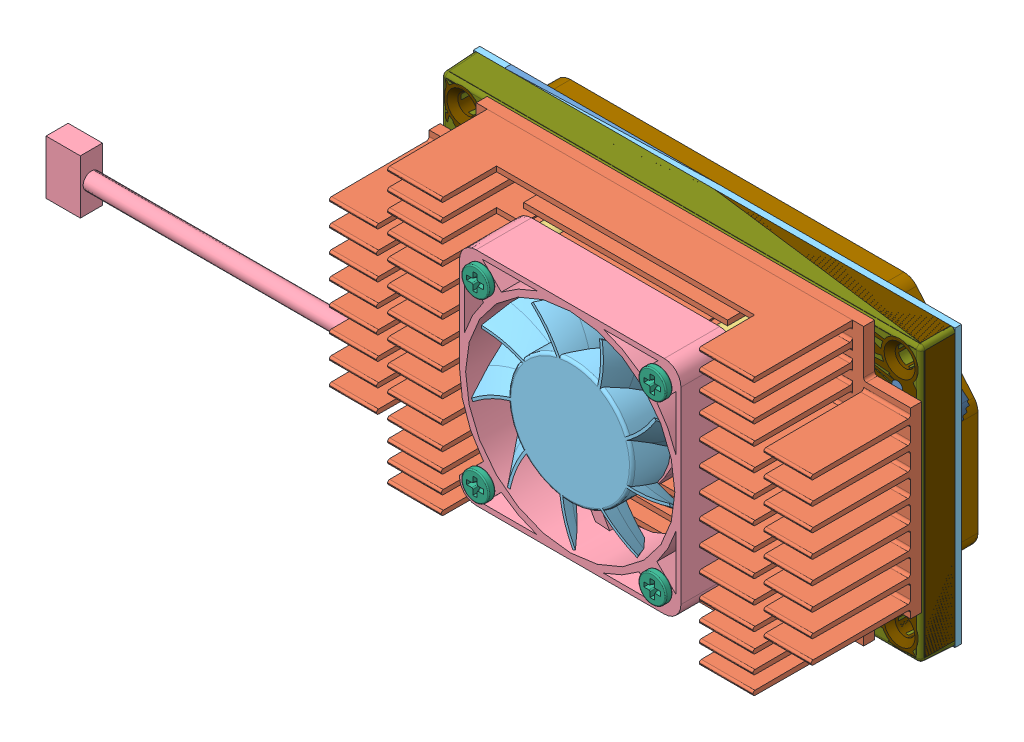
SolidWorks assembly JETSON-NEW_ASM, configuration Default. Lengths in mm. (continued)
Components (placement in the parent): (continued)
- 244-82180-1000-A03-10-12-15_ASM-1: 244-82180-1000-A03-10-12-15_ASM [Default] at origin size (87 50 8.3) (continued)
  - 195-2319-000_1-2: 195-2319-000_1 [Default] at (56.55 19.856 0) x (0 -1 0) z (0 0 -1) size (0.69 0.32 0.31)
  - 195-2299-000_1-2: 195-2299-000_1 [Default] at (58.55 21.116 0) x (-1 0 0) z (0 0 -1) size (0.69 0.32 0.31)
  - 195-2289-000_1-2: 195-2289-000_1 [Default] at (57.09 19.856 0) x (0 1 0) z (0 0 -1) size (0.69 0.32 0.31)
  - 195-1636-000_1-101: 195-1636-000_1 [Default] at (58.55 21.656 0) x (1 0 0) z (0 0 -1) size (0.69 0.32 0.31)
  - 032-0335-000_1-2: 032-0335-000_1 [Default] at (58.55 20.576 0) x (-1 0 0) z (0 0 -1) size (0.69 0.32 0.34)
  - 039-0199-000_1-3: 039-0199-000_1 [Default] at (57.63 19.856 0) x (0 1 0) z (0 0 -1) size (0.69 0.32 0.36)
  - 039-0204-000_1-1: 039-0204-000_1 [Default] at (71.45 25.1 0) x (-1 0 0) z (0 0 -1) size (0.69 0.32 0.34)
  - 039-0204-000_1-2: 039-0204-000_1 [Default] at (58.17 19.856 0) x (0 1 0) z (0 0 -1) size (0.69 0.32 0.34)
  - 195-1636-000_1-102: 195-1636-000_1 [Default] at (71.453 24.573 0) x (1 0 0) z (0 0 -1) size (0.69 0.32 0.31)
  - 195-1636-000_1-103: 195-1636-000_1 [Default] at (58.74 19.856 0) x (0 -1 0) z (0 0 -1) size (0.69 0.32 0.31)
  - 101-0142-000_2-1: 101-0142-000_2 [Default] at (6.063 36.964 1.164) x (0 1 0) z (0 0 1) size (1.4 1.1 0.4)
  - 101-0142-000_2-2: 101-0142-000_2 [Default] at (5.31 31.454 1.164) x (0 1 0) z (0 0 1) size (1.4 1.1 0.4)
  - 085-0203-000_1-1: 085-0203-000_1 [Default] at (13.653 29.754 1.164) size (1.75 1.35 0.4)
  - 131-0802-000_2-1: 131-0802-000_2 [Default] at (18.469 28.798 1.164) x (0 -1 0) z (0 0 1) size (2.53 1.61 1.01)
  - 085-0180-000_1-1: 085-0180-000_1 [Default] at (23.25 23 1.164) x (-1 0 0) z (0 0 1) size (2.9 2.5 0.56)
  - 305-0057-000_1-1: 305-0057-000_1 [Default] at (41.153 40.254 0) x (1 0 0) z (0 0 -1) size (2 2.69 1.1)
  - 115-0057-000_1-1: 115-0057-000_1 [Default] at (5.8 35.45 0) x (0 1 0) z (0 0 -1) size (2 2.88 1.1)
  - 115-1572-000_1-1: 115-1572-000_1 [Default] at (65.88 15.256 0) x (0 -1 0) z (0 0 -1) size (2 2.88 1.1)
  - 315-0217-000_1-1: 315-0217-000_1 [Default] at (41.273 36.727 0) x (1 0 0) z (0 0 -1) size (2 2.88 1.1)
  - 130-0646-000_1-1: 130-0646-000_1 [Default] at (57.753 23.554 1.164) x (-1 0 0) z (0 0 1) size (8.4 6.6 1.8)
  - 130-0646-000_1-2: 130-0646-000_1 [Default] at (57.753 16.304 1.164) x (-1 0 0) z (0 0 1) size (8.4 6.6 1.8)
  - 130-0562-000_2-1: 130-0562-000_2 [Default] at (56.978 30.96 1.164) x (0 -1 0) z (0 0 1) size (2.8 2.25 1.22)
  - 130-0562-000_2-2: 130-0562-000_2 [Default] at (53.858 37.854 1.164) x (0 1 0) z (0 0 1) size (2.8 2.25 1.22)
  - 130-0562-000_2-3: 130-0562-000_2 [Default] at (53.848 33.894 1.164) x (0 -1 0) z (0 0 1) size (2.8 2.25 1.22)
  - 130-0562-000_2-4: 130-0562-000_2 [Default] at (59.478 30.965 1.164) x (0 -1 0) z (0 0 1) size (2.8 2.25 1.22)
  - 130-0562-000_2-5: 130-0562-000_2 [Default] at (63.578 33.764 1.164) x (0 -1 0) z (0 0 1) size (2.8 2.25 1.22)
  - 300-0252-000_1-1: 300-0252-000_1 [Default] at (63.7 17.8 1.164) x (0 -1 0) z (0 0 1) size (3.81 3.5 0.81)
  - 300-0252-000_1-2: 300-0252-000_1 [Default] at (63.7 22.25 1.164) x (0 1 0) z (0 0 1) size (3.81 3.5 0.81)
  - 300-0252-000_1-3: 300-0252-000_1 [Default] at (63.7 13.55 1.164) x (0 1 0) z (0 0 1) size (3.81 3.5 0.81)
  - 300-0252-000_1-4: 300-0252-000_1 [Default] at (63.7 26.5 1.164) x (0 -1 0) z (0 0 1) size (3.81 3.5 0.81)
  - 300-0284-000_1-1: 300-0284-000_1 [Default] at (67.9 22.7 1.164) size (3.81 3.5 0.81)
  - 300-0284-000_1-2: 300-0284-000_1 [Default] at (67.9 15.45 1.164) size (3.81 3.5 0.81)
  - 195-0487-000_1-1: 195-0487-000_1 [Default] at (63.7 12.3 0) x (0 -1 0) z (0 0 -1) size (1.2 0.5 0.4)
  - 039-0208-000_1-1: 039-0208-000_1 [Default] at (4.01 9.61 1.164) x (0 1 0) z (0 0 1) size (1.2 0.5 0.55)
  - 039-0208-000_1-2: 039-0208-000_1 [Default] at (73.36 37.97 1.164) size (1.2 0.5 0.55)
  - 032-0204-000_2-1: 032-0204-000_2 [Default] at (69.95 26.3 0) x (0 1 0) z (0 0 -1) size (1.2 0.5 0.55)
  - 195-0486-000_1-1: 195-0486-000_1 [Default] at (9.75 33.6 0) x (-1 0 0) z (0 0 -1) size (1.2 0.5 0.4)
  - 195-0324-000_1-1: 195-0324-000_1 [Default] at (10.2 30.95 0) x (0 -1 0) z (0 0 -1) size (1.2 0.5 0.4)
  - 195-0235-000_1-1: 195-0235-000_1 [Default] at (9.4 32.45 0) x (0 -1 0) z (0 0 -1) size (1.2 0.5 0.4)
  - 036-0014-000_1-1: 036-0014-000_1 [Default] at (6.25 30.3 0) x (1 0 0) z (0 0 -1) size (1.2 0.5 0.6)
  - 036-0014-000_1-2: 036-0014-000_1 [Default] at (9.4 30.95 0) x (0 -1 0) z (0 0 -1) size (1.2 0.5 0.6)
  - 195-1691-000_1-1: 195-1691-000_1 [Default] at (44.62 11.876 0) x (0 1 0) z (0 0 -1) size (1.2 0.5 0.4)
  - 195-1691-000_1-2: 195-1691-000_1 [Default] at (43.89 11.876 0) x (0 1 0) z (0 0 -1) size (1.2 0.5 0.4)
  - 195-0415-000_1-1: 195-0415-000_1 [Default] at (74.79 39.5 1.164) x (0 1 0) z (0 0 1) size (1.2 0.5 0.4)
  - 035-0017-000_1-1: 035-0017-000_1 [Default] at (76.18 34.056 1.164) x (0 -1 0) z (0 0 1) size (1.2 0.5 0.6)
  - 195-0210-000_1-1: 195-0210-000_1 [Default] at (77.99 35.336 1.164) size (1.2 0.5 0.4)
  - 195-0475-000_1-1: 195-0475-000_1 [Default] at (77.98 34.596 1.164) x (-1 0 0) z (0 0 1) size (1.2 0.5 0.4)
  - 036-0141-000_1-1: 036-0141-000_1 [Default] at (76.93 34.056 1.164) x (0 -1 0) z (0 0 1) size (1.2 0.5 0.61)
  - 195-0070-000_1-1: 195-0070-000_1 [Default] at (76.53 35.156 1.164) size (1.2 0.5 0.4)
  - 035-0212-000_1-1: 035-0212-000_1 [Default] at (77.69 32.384 1.164) x (0 1 0) z (0 0 1) size (1.2 0.5 0.55)
  - 195-0005-000_1-1: 195-0005-000_1 [Default] at (76.97 32.384 1.164) x (0 1 0) z (0 0 1) size (1.2 0.5 0.4)
  - 195-0140-000_1-1: 195-0140-000_1 [Default] at (75.74 32.814 1.164) x (-1 0 0) z (0 0 1) size (1.2 0.5 0.4)
  - 195-0342-000_1-1: 195-0342-000_1 [Default] at (75.776 31.96 1.164) size (1.2 0.5 0.4)
  - 195-0405-000_1-1: 195-0405-000_1 [Default] at (2.04 14.56 1.164) x (-1 0 0) z (0 0 1) size (1.2 0.5 0.4)
  - 035-0212-000_1-2: 035-0212-000_1 [Default] at (8.776 12.06 1.164) x (0 -1 0) z (0 0 1) size (1.2 0.5 0.55)
  - 195-0487-000_1-2: 195-0487-000_1 [Default] at (0.85 14.75 1.164) x (0 1 0) z (0 0 1) size (1.2 0.5 0.4)
  - 195-0240-000_1-1: 195-0240-000_1 [Default] at (0.1 14.75 1.164) x (0 -1 0) z (0 0 1) size (1.2 0.5 0.4)
  - 036-0141-000_1-2: 036-0141-000_1 [Default] at (9.126 10.96 1.164) x (-1 0 0) z (0 0 1) size (1.2 0.5 0.61)
  - 195-0404-000_1-1: 195-0404-000_1 [Default] at (9.526 12.06 1.164) x (0 -1 0) z (0 0 1) size (1.2 0.5 0.4)
  - 035-0212-000_1-3: 035-0212-000_1 [Default] at (10.24 9.756 1.164) x (0 -1 0) z (0 0 1) size (1.2 0.5 0.55)
  - 195-0342-000_1-2: 195-0342-000_1 [Default] at (11.404 10.18 1.164) x (-1 0 0) z (0 0 1) size (1.2 0.5 0.4)
  - 195-0005-000_1-2: 195-0005-000_1 [Default] at (9.53 9.756 1.164) x (0 -1 0) z (0 0 1) size (1.2 0.5 0.4)
  - 195-0250-000_1-1: 195-0250-000_1 [Default] at (8.664 9.78 1.164) x (0 1 0) z (0 0 1) size (1.2 0.5 0.4)
  - 195-0485-000_1-1: 195-0485-000_1 [Default] at (5.7 11.85 0) x (-1 0 0) z (0 0 -1) size (1.2 0.5 0.4)
  - 195-0485-000_1-2: 195-0485-000_1 [Default] at (5.7 12.6 0) x (-1 0 0) z (0 0 -1) size (1.2 0.5 0.4)
  - 039-0023-000_1-1: 039-0023-000_1 [Default] at (36.871 31.058 0) x (-1 0 0) z (0 0 -1) size (1.2 0.5 0.6)
  - 195-0031-000_1-1: 195-0031-000_1 [Default] at (35.801 30.61 0) x (0 1 0) z (0 0 -1) size (1.2 0.5 0.4)
  - 195-2655-000_1-1: 195-2655-000_1 [Default] at (36.871 30.308 0) x (-1 0 0) z (0 0 -1) size (1.2 0.5 0.4)
  - 195-0437-000_1-1: 195-0437-000_1 [Default] at (36.479 24.219 0) x (0 -1 0) z (0 0 -1) size (1.2 0.5 0.4)
  - 195-0292-000_1-1: 195-0292-000_1 [Default] at (35.427 24.921 0) x (-1 0 0) z (0 0 -1) size (1.2 0.5 0.4)
  - 039-0008-000_1-1: 039-0008-000_1 [Default] at (39.63 37.104 0) x (0 -1 0) z (0 0 -1) size (1.2 0.5 0.6)
  - 039-0008-000_1-2: 039-0008-000_1 [Default] at (41.103 34.754 0) x (1 0 0) z (0 0 -1) size (1.2 0.5 0.6)
  - 195-0484-000_1-1: 195-0484-000_1 [Default] at (46.963 29.024 0) x (1 0 0) z (0 0 -1) size (1.2 0.5 0.4)
  - 195-0596-000_1-1: 195-0596-000_1 [Default] at (46.963 28.214 0) x (1 0 0) z (0 0 -1) size (1.2 0.5 0.4)
  - 195-0002-000_1-1: 195-0002-000_1 [Default] at (52.188 28.414 0) x (-1 0 0) z (0 0 -1) size (1.2 0.5 0.4)
  - 036-0012-000_1-1: 036-0012-000_1 [Default] at (51.053 28.084 0) x (0 -1 0) z (0 0 -1) size (1.2 0.5 0.6)
  - 195-0486-000_1-2: 195-0486-000_1 [Default] at (69.45 10.95 1.164) size (1.2 0.5 0.4)
  - 039-0008-000_1-3: 039-0008-000_1 [Default] at (11.5 19.1 0) x (0 -1 0) z (0 0 -1) size (1.2 0.5 0.6)
  - 195-2655-000_1-2: 195-2655-000_1 [Default] at (19.934 31.265 0) x (0 -1 0) z (0 0 -1) size (1.2 0.5 0.4)
  - 039-0008-000_1-4: 039-0008-000_1 [Default] at (21.486 32.341 0) x (-1 0 0) z (0 0 -1) size (1.2 0.5 0.6)
  - 195-2655-000_1-3: 195-2655-000_1 [Default] at (20.641 31.27 0) x (0 -1 0) z (0 0 -1) size (1.2 0.5 0.4)
  - 039-0136-000_1-1: 039-0136-000_1 [Default] at (10.606 31.182 1.164) x (-0.707107 -0.707107 0) z (0 0 1) size (1.2 0.5 0.61)
  - 039-0136-000_1-2: 039-0136-000_1 [Default] at (12.104 29.849 1.164) x (0 1 0) z (0 0 1) size (1.2 0.5 0.61)
  - 039-0136-000_1-3: 039-0136-000_1 [Default] at (11.729 28.799 1.164) x (-1 0 0) z (0 0 1) size (1.2 0.5 0.61)
  - 039-0136-000_1-4: 039-0136-000_1 [Default] at (14.693 27.88 1.164) x (-1 0 0) z (0 0 1) size (1.2 0.5 0.61)
  - 039-0136-000_1-5: 039-0136-000_1 [Default] at (12.197 36.147 1.164) x (-1 0 0) z (0 0 1) size (1.2 0.5 0.61)
  - 039-0008-000_1-5: 039-0008-000_1 [Default] at (13.012 34.245 0) x (0 1 0) z (0 0 -1) size (1.2 0.5 0.6)
  - 195-2655-000_1-4: 195-2655-000_1 [Default] at (13.563 33.192 0) x (1 0 0) z (0 0 -1) size (1.2 0.5 0.4)
  - 039-0136-000_1-6: 039-0136-000_1 [Default] at (13.208 27.925 1.164) x (-1 0 0) z (0 0 1) size (1.2 0.5 0.61)
  - 195-2655-000_1-5: 195-2655-000_1 [Default] at (18.836 32.716 0) x (0 -1 0) z (0 0 -1) size (1.2 0.5 0.4)
  - 032-0153-000_2-1: 032-0153-000_2 [Default] at (17.436 32.716 0) x (0 1 0) z (0 0 -1) size (1.2 0.5 0.6)
  - 039-0008-000_1-6: 039-0008-000_1 [Default] at (14.75 39.45 0) x (-1 0 0) z (0 0 -1) size (1.2 0.5 0.6)
  - 195-2655-000_1-6: 195-2655-000_1 [Default] at (15.15 38.25 0) x (0 1 0) z (0 0 -1) size (1.2 0.5 0.4)
  - 039-0008-000_1-7: 039-0008-000_1 [Default] at (15.15 42.05 0) x (0 1 0) z (0 0 -1) size (1.2 0.5 0.6)
  - 039-0136-000_1-7: 039-0136-000_1 [Default] at (16.088 35.815 0) x (0 1 0) z (0 0 -1) size (1.2 0.5 0.61)
  - 039-0136-000_1-8: 039-0136-000_1 [Default] at (16.036 33.333 0) x (0 1 0) z (0 0 -1) size (1.2 0.5 0.61)
  - 039-0008-000_1-8: 039-0008-000_1 [Default] at (17.786 33.809 0) x (1 0 0) z (0 0 -1) size (1.2 0.5 0.6)
  - 039-0011-000_1-1: 039-0011-000_1 [Default] at (16.736 32.933 0) x (0 1 0) z (0 0 -1) size (1.2 0.5 0.6)
  - 039-0136-000_1-9: 039-0136-000_1 [Default] at (15.842 29.849 1.164) x (0 -1 0) z (0 0 1) size (1.2 0.5 0.61)
  - 032-0153-000_2-2: 032-0153-000_2 [Default] at (17.068 29.641 1.164) x (0 -1 0) z (0 0 1) size (1.2 0.5 0.6)
  - 195-2655-000_1-7: 195-2655-000_1 [Default] at (27.6 19.65 0) x (0 -1 0) z (0 0 -1) size (1.2 0.5 0.4)
  - 039-0008-000_1-9: 039-0008-000_1 [Default] at (26.268 14.214 0) x (0 1 0) z (0 0 -1) size (1.2 0.5 0.6)
  - 195-2655-000_1-8: 195-2655-000_1 [Default] at (24.438 17.784 0) x (1 0 0) z (0 0 -1) size (1.2 0.5 0.4)
  - 039-0008-000_1-10: 039-0008-000_1 [Default] at (25.473 16.544 0) x (0 -1 0) z (0 0 -1) size (1.2 0.5 0.6)
  - 039-0008-000_1-11: 039-0008-000_1 [Default] at (25.032 13.913 0) x (1 0 0) z (0 0 -1) size (1.2 0.5 0.6)
  - 039-0008-000_1-12: 039-0008-000_1 [Default] at (23.442 16.554 0) x (0 -1 0) z (0 0 -1) size (1.2 0.5 0.6)
  - 039-0008-000_1-13: 039-0008-000_1 [Default] at (33.563 14.704 0) x (0 1 0) z (0 0 -1) size (1.2 0.5 0.6)
  - 039-0008-000_1-14: 039-0008-000_1 [Default] at (39.241 18.025 0) x (1 0 0) z (0 0 -1) size (1.2 0.5 0.6)
  - 039-0008-000_1-15: 039-0008-000_1 [Default] at (37.923 13.224 0) x (0 -1 0) z (0 0 -1) size (1.2 0.5 0.6)
  - 039-0008-000_1-16: 039-0008-000_1 [Default] at (36.533 21.324 0) x (0 -1 0) z (0 0 -1) size (1.2 0.5 0.6)
  - 039-0008-000_1-17: 039-0008-000_1 [Default] at (36.883 19.644 0) x (0 -1 0) z (0 0 -1) size (1.2 0.5 0.6)
  - 039-0008-000_1-18: 039-0008-000_1 [Default] at (36.423 14.689 0) x (0 -1 0) z (0 0 -1) size (1.2 0.5 0.6)
  - 039-0008-000_1-19: 039-0008-000_1 [Default] at (34.543 20.894 0) x (-1 0 0) z (0 0 -1) size (1.2 0.5 0.6)
  - 039-0008-000_1-20: 039-0008-000_1 [Default] at (43.6 19.15 0) x (0 1 0) z (0 0 -1) size (1.2 0.5 0.6)
  - 039-0008-000_1-21: 039-0008-000_1 [Default] at (34.282 15.951 0) x (0 1 0) z (0 0 -1) size (1.2 0.5 0.6)
  - 039-0008-000_1-22: 039-0008-000_1 [Default] at (39.653 19.654 0) x (0 -1 0) z (0 0 -1) size (1.2 0.5 0.6)
  - 039-0008-000_1-23: 039-0008-000_1 [Default] at (40.423 13.214 0) x (0 -1 0) z (0 0 -1) size (1.2 0.5 0.6)
  - 195-2655-000_1-9: 195-2655-000_1 [Default] at (39.163 11.574 0) x (0 1 0) z (0 0 -1) size (1.2 0.5 0.4)
  - 035-0012-000_1-1: 035-0012-000_1 [Default] at (66.85 13.326 0) x (0 -1 0) z (0 0 -1) size (1.2 0.5 0.6)
  - 195-0315-000_1-1: 195-0315-000_1 [Default] at (66.1 13.326 0) x (0 -1 0) z (0 0 -1) size (1.2 0.5 0.4)
  - 195-0005-000_1-3: 195-0005-000_1 [Default] at (65.35 13.326 0) x (0 -1 0) z (0 0 -1) size (1.2 0.5 0.4)
  - 195-0200-000_1-1: 195-0200-000_1 [Default] at (69.4 15.1 0) x (0 1 0) z (0 0 -1) size (1.2 0.5 0.4)
  - 039-0008-000_1-24: 039-0008-000_1 [Default] at (43.95 20.2 0) x (1 0 0) z (0 0 -1) size (1.2 0.5 0.6)
  - 195-2655-000_1-10: 195-2655-000_1 [Default] at (65.838 16.894 0) x (1 0 0) z (0 0 -1) size (1.2 0.5 0.4)
  - 039-0008-000_1-25: 039-0008-000_1 [Default] at (46.11 16.806 1.164) x (0 -1 0) z (0 0 1) size (1.2 0.5 0.6)
  - 039-0008-000_1-26: 039-0008-000_1 [Default] at (44.65 19.1 0) x (0 1 0) z (0 0 -1) size (1.2 0.5 0.6)
  - 195-0485-000_1-3: 195-0485-000_1 [Default] at (50.55 26.4 0) x (0 1 0) z (0 0 -1) size (1.2 0.5 0.4)
  - 195-0485-000_1-4: 195-0485-000_1 [Default] at (49.85 26.4 0) x (0 1 0) z (0 0 -1) size (1.2 0.5 0.4)
  - 195-0005-000_1-4: 195-0005-000_1 [Default] at (68.7 15.1 0) x (0 1 0) z (0 0 -1) size (1.2 0.5 0.4)
  - 039-0008-000_1-27: 039-0008-000_1 [Default] at (45.55 21.7 1.164) x (-1 0 0) z (0 0 1) size (1.2 0.5 0.6)
  - 039-0008-000_1-28: 039-0008-000_1 [Default] at (45.36 16.806 1.164) x (0 -1 0) z (0 0 1) size (1.2 0.5 0.6)
  - 036-0014-000_1-3: 036-0014-000_1 [Default] at (59.75 19.766 0) x (1 0 0) z (0 0 -1) size (1.2 0.5 0.6)
  - 039-0008-000_1-29: 039-0008-000_1 [Default] at (57.013 39.939 1.164) x (0 -1 0) z (0 0 1) size (1.2 0.5 0.6)
  - 039-0136-000_1-10: 039-0136-000_1 [Default] at (57.028 38.454 1.164) x (0 1 0) z (0 0 1) size (1.2 0.5 0.61)
  - 039-0008-000_1-30: 039-0008-000_1 [Default] at (56.232 38.857 0) x (-1 0 0) z (0 0 -1) size (1.2 0.5 0.6)
  - 195-0004-000_1-1: 195-0004-000_1 [Default] at (57.463 14.604 0) x (0 -1 0) z (0 0 -1) size (1.2 0.5 0.4)
  - 036-0014-000_1-4: 036-0014-000_1 [Default] at (56.423 15.284 0) x (0 -1 0) z (0 0 -1) size (1.2 0.5 0.6)
  - 036-0212-000_2-1: 036-0212-000_2 [Default] at (53.353 13.204 1.164) x (0 1 0) z (0 0 1) size (1.2 0.5 0.61)
  - 195-0150-000_1-1: 195-0150-000_1 [Default] at (53.353 11.704 1.164) x (0 1 0) z (0 0 1) size (1.2 0.5 0.4)
  - 039-0008-000_1-31: 039-0008-000_1 [Default] at (59.828 38.454 1.164) x (0 1 0) z (0 0 1) size (1.2 0.5 0.6)
  - 039-0008-000_1-32: 039-0008-000_1 [Default] at (60.528 38.454 1.164) x (0 1 0) z (0 0 1) size (1.2 0.5 0.6)
  - 039-0136-000_1-11: 039-0136-000_1 [Default] at (61.1 38.2 0) x (0 1 0) z (0 0 -1) size (1.2 0.5 0.61)
  - 039-0008-000_1-33: 039-0008-000_1 [Default] at (59.353 36.004 0) x (0 -1 0) z (0 0 -1) size (1.2 0.5 0.6)
  - 039-0008-000_1-34: 039-0008-000_1 [Default] at (60.303 36.904 0) x (0 -1 0) z (0 0 -1) size (1.2 0.5 0.6)
  - 195-0542-000_1-1: 195-0542-000_1 [Default] at (59.753 22.304 0) x (1 0 0) z (0 0 -1) size (1.2 0.5 0.4)
  - 195-0379-000_1-1: 195-0379-000_1 [Default] at (59.753 21.544 0) x (1 0 0) z (0 0 -1) size (1.2 0.5 0.4)
  - 195-2655-000_1-11: 195-2655-000_1 [Default] at (60.853 22.004 0) x (0 1 0) z (0 0 -1) size (1.2 0.5 0.4)
  - 195-0004-000_1-2: 195-0004-000_1 [Default] at (59.75 20.516 0) x (1 0 0) z (0 0 -1) size (1.2 0.5 0.4)
  - 195-0004-000_1-3: 195-0004-000_1 [Default] at (60.853 20.404 0) x (0 1 0) z (0 0 -1) size (1.2 0.5 0.4)
  - 195-0595-000_1-1: 195-0595-000_1 [Default] at (59.403 14.104 0) x (0 1 0) z (0 0 -1) size (1.2 0.5 0.4)
  - 039-0008-000_1-35: 039-0008-000_1 [Default] at (59.128 38.454 1.164) x (0 1 0) z (0 0 1) size (1.2 0.5 0.6)
  - 039-0008-000_1-36: 039-0008-000_1 [Default] at (58.3 40.45 0) x (0 -1 0) z (0 0 -1) size (1.2 0.5 0.6)
  - 039-0008-000_1-37: 039-0008-000_1 [Default] at (57.713 39.939 1.164) x (0 -1 0) z (0 0 1) size (1.2 0.5 0.6)
  - 039-0008-000_1-38: 039-0008-000_1 [Default] at (58.428 38.454 1.164) x (0 1 0) z (0 0 1) size (1.2 0.5 0.6)
  - 039-0008-000_1-39: 039-0008-000_1 [Default] at (57.728 38.454 1.164) x (0 1 0) z (0 0 1) size (1.2 0.5 0.6)
  - 035-0023-000_1-1: 035-0023-000_1 [Default] at (62.753 19.154 0) x (1 0 0) z (0 0 -1) size (1.2 0.5 0.6)
  - 195-0150-000_1-2: 195-0150-000_1 [Default] at (61.8 23.85 0) x (1 0 0) z (0 0 -1) size (1.2 0.5 0.4)
  - 036-0212-000_2-2: 036-0212-000_2 [Default] at (61.8 23.1 0) x (-1 0 0) z (0 0 -1) size (1.2 0.5 0.61)
  - 195-2655-000_1-12: 195-2655-000_1 [Default] at (62.253 22.004 0) x (0 1 0) z (0 0 -1) size (1.2 0.5 0.4)
  - 036-0012-000_1-2: 036-0012-000_1 [Default] at (61.553 22.004 0) x (0 1 0) z (0 0 -1) size (1.2 0.5 0.6)
  - 195-2655-000_1-13: 195-2655-000_1 [Default] at (62.253 20.404 0) x (0 1 0) z (0 0 -1) size (1.2 0.5 0.4)
  - 035-0023-000_1-2: 035-0023-000_1 [Default] at (61.553 20.404 0) x (0 1 0) z (0 0 -1) size (1.2 0.5 0.6)
  - 035-0023-000_1-3: 035-0023-000_1 [Default] at (61.303 19.154 0) x (1 0 0) z (0 0 -1) size (1.2 0.5 0.6)
  - 036-0021-000_1-1: 036-0021-000_1 [Default] at (62.503 18.054 0) x (0 -1 0) z (0 0 -1) size (1.2 0.5 0.6)
  - 035-0023-000_1-4: 035-0023-000_1 [Default] at (61.103 18.054 0) x (0 1 0) z (0 0 -1) size (1.2 0.5 0.6)
  - 195-0105-000_1-1: 195-0105-000_1 [Default] at (61.803 18.054 0) x (0 1 0) z (0 0 -1) size (1.2 0.5 0.4)
  - 195-2655-000_1-14: 195-2655-000_1 [Default] at (63.1 37.45 0) x (0 -1 0) z (0 0 -1) size (1.2 0.5 0.4)
  - 195-0004-000_1-4: 195-0004-000_1 [Default] at (65.593 23.204 0) x (-1 0 0) z (0 0 -1) size (1.2 0.5 0.4)
  - 195-0595-000_1-2: 195-0595-000_1 [Default] at (65.204 20.979 0) x (0 1 0) z (0 0 -1) size (1.2 0.5 0.4)
  - 195-0003-000_1-1: 195-0003-000_1 [Default] at (63.3 18.05 0) x (0 -1 0) z (0 0 -1) size (1.2 0.5 0.4)
  - 035-0023-000_1-5: 035-0023-000_1 [Default] at (64.2 18.05 0) x (0 1 0) z (0 0 -1) size (1.2 0.5 0.6)
  - 195-0220-000_1-1: 195-0220-000_1 [Default] at (64.28 31.616 0) x (1 0 0) z (0 0 -1) size (1.2 0.5 0.4)
  - 195-0031-000_1-2: 195-0031-000_1 [Default] at (65.71 31.026 0) x (1 0 0) z (0 0 -1) size (1.2 0.5 0.4)
  - 036-0014-000_1-5: 036-0014-000_1 [Default] at (67.353 24.804 0) x (0 1 0) z (0 0 -1) size (1.2 0.5 0.6)
  - 039-0028-000_1-1: 039-0028-000_1 [Default] at (66.69 24.97 1.164) x (-1 0 0) z (0 0 1) size (1.2 0.5 0.6)
  - 039-0028-000_1-2: 039-0028-000_1 [Default] at (67.1 13.1 1.164) x (-1 0 0) z (0 0 1) size (1.2 0.5 0.6)
  - 039-0028-000_1-3: 039-0028-000_1 [Default] at (67.3 17.85 1.164) x (-1 0 0) z (0 0 1) size (1.2 0.5 0.6)
  - 039-0028-000_1-4: 039-0028-000_1 [Default] at (68.5 20.35 1.164) x (-1 0 0) z (0 0 1) size (1.2 0.5 0.6)
  - 039-0008-000_1-40: 039-0008-000_1 [Default] at (12.15 20.55 0) x (0 -1 0) z (0 0 -1) size (1.2 0.5 0.6)
  - 035-0011-000_1-1: 035-0011-000_1 [Default] at (25.25 21.95 1.164) x (0 -1 0) z (0 0 1) size (1.2 0.5 0.6)
  - 035-0011-000_1-2: 035-0011-000_1 [Default] at (25.25 23.5 1.164) x (0 -1 0) z (0 0 1) size (1.2 0.5 0.6)
  - 195-0002-000_1-2: 195-0002-000_1 [Default] at (52.188 27.614 0) x (-1 0 0) z (0 0 -1) size (1.2 0.5 0.4)
  - 039-0008-000_1-41: 039-0008-000_1 [Default] at (40.023 22.324 0) x (0 -1 0) z (0 0 -1) size (1.2 0.5 0.6)
  - 195-0002-000_1-3: 195-0002-000_1 [Default] at (64.61 19.117 0) x (-1 0 0) z (0 0 -1) size (1.2 0.5 0.4)
  - 195-0002-000_1-4: 195-0002-000_1 [Default] at (63.3 22 0) x (0 1 0) z (0 0 -1) size (1.2 0.5 0.4)
  - 195-2655-000_1-15: 195-2655-000_1 [Default] at (63.3 20.4 0) x (0 1 0) z (0 0 -1) size (1.2 0.5 0.4)
  - 195-2655-000_1-16: 195-2655-000_1 [Default] at (64.1 20.4 0) x (0 -1 0) z (0 0 -1) size (1.2 0.5 0.4)
  - 195-0194-000_1-1: 195-0194-000_1 [Default] at (70.17 6.58 1.164) x (-1 0 0) z (0 0 1) size (1.2 0.5 0.4)
  - 195-0486-000_1-3: 195-0486-000_1 [Default] at (75.11 13.02 1.164) size (1.2 0.5 0.4)
  - 195-0486-000_1-4: 195-0486-000_1 [Default] at (69.45 10.2 1.164) size (1.2 0.5 0.4)
  - 195-0486-000_1-5: 195-0486-000_1 [Default] at (69.45 11.65 1.164) size (1.2 0.5 0.4)
  - 195-0005-000_1-5: 195-0005-000_1 [Default] at (68.65 16.75 0) x (0 1 0) z (0 0 -1) size (1.2 0.5 0.4)
  - 195-0005-000_1-6: 195-0005-000_1 [Default] at (73.7 14.1 0) x (0 1 0) z (0 0 -1) size (1.2 0.5 0.4)
  - 195-2655-000_1-17: 195-2655-000_1 [Default] at (75.15 14.6 1.164) size (1.2 0.5 0.4)
  - 195-2655-000_1-18: 195-2655-000_1 [Default] at (69.4 16.75 0) x (0 1 0) z (0 0 -1) size (1.2 0.5 0.4)
  - 036-0014-000_1-6: 036-0014-000_1 [Default] at (70.17 7.3 1.164) x (-1 0 0) z (0 0 1) size (1.2 0.5 0.6)
  - 035-0026-000_1-1: 035-0026-000_1 [Default] at (68.34 7.2 1.164) x (0 -1 0) z (0 0 1) size (1.2 0.5 0.6)
  - 035-0026-000_1-2: 035-0026-000_1 [Default] at (68.34 8.65 1.164) x (0 1 0) z (0 0 1) size (1.2 0.5 0.6)
  - 036-0014-000_1-7: 036-0014-000_1 [Default] at (71.15 5.1 1.164) x (-1 0 0) z (0 0 1) size (1.2 0.5 0.6)
  - 036-0014-000_1-8: 036-0014-000_1 [Default] at (69.45 8.75 1.164) x (-1 0 0) z (0 0 1) size (1.2 0.5 0.6)
  - 036-0014-000_1-9: 036-0014-000_1 [Default] at (74.05 13.37 1.164) x (0 1 0) z (0 0 1) size (1.2 0.5 0.6)
  - 036-0014-000_1-10: 036-0014-000_1 [Default] at (75.11 13.77 1.164) x (-1 0 0) z (0 0 1) size (1.2 0.5 0.6)
  - 036-0014-000_1-11: 036-0014-000_1 [Default] at (76.56 13.02 1.164) size (1.2 0.5 0.6)
  - 039-0008-000_1-42: 039-0008-000_1 [Default] at (76.56 13.77 1.164) size (1.2 0.5 0.6)
  - 036-0014-000_1-12: 036-0014-000_1 [Default] at (78.1 12.55 1.164) size (1.2 0.5 0.6)
  - 036-0014-000_1-13: 036-0014-000_1 [Default] at (78.13 11 1.164) size (1.2 0.5 0.6)
  - 036-0014-000_1-14: 036-0014-000_1 [Default] at (78.13 6.08 1.164) size (1.2 0.5 0.6)
  - 036-0014-000_1-15: 036-0014-000_1 [Default] at (78.1 9.9 1.164) size (1.2 0.5 0.6)
  - 036-0014-000_1-16: 036-0014-000_1 [Default] at (75.55 5.1 1.164) size (1.2 0.5 0.6)
  - 036-0014-000_1-17: 036-0014-000_1 [Default] at (70 5.45 1.164) x (0 -1 0) z (0 0 1) size (1.2 0.5 0.6)
  - 036-0014-000_1-18: 036-0014-000_1 [Default] at (78.13 11.75 1.164) size (1.2 0.5 0.6)
  - 036-0014-000_1-19: 036-0014-000_1 [Default] at (78.13 5.33 1.164) size (1.2 0.5 0.6)
  - 036-0014-000_1-20: 036-0014-000_1 [Default] at (78.13 7.57 1.164) x (-1 0 0) z (0 0 1) size (1.2 0.5 0.6)
  - 036-0014-000_1-21: 036-0014-000_1 [Default] at (78.13 6.83 1.164) x (-1 0 0) z (0 0 1) size (1.2 0.5 0.6)
  - 036-0014-000_1-22: 036-0014-000_1 [Default] at (78.13 9.17 1.164) x (-1 0 0) z (0 0 1) size (1.2 0.5 0.6)
  - 036-0014-000_1-23: 036-0014-000_1 [Default] at (78.13 8.43 1.164) x (-1 0 0) z (0 0 1) size (1.2 0.5 0.6)
  - 036-0014-000_1-24: 036-0014-000_1 [Default] at (72.75 5.1 1.164) x (-1 0 0) z (0 0 1) size (1.2 0.5 0.6)
  - 039-0008-000_1-43: 039-0008-000_1 [Default] at (69.95 9.45 1.164) x (-1 0 0) z (0 0 1) size (1.2 0.5 0.6)
  - 195-0489-000_1-1: 195-0489-000_1 [Default] at (63.7 13.8 0) x (0 1 0) z (0 0 -1) size (1.2 0.5 0.4)
  - 039-0188-000_3-1: 039-0188-000_3 [Default] at (30.85 35.8 0) x (-1 0 0) z (0 0 -1) size (1.4 0.7 0.67)
  - 039-0145-000_2-1: 039-0145-000_2 [Default] at (75.7 33.7 0) x (0 1 0) z (0 0 -1) size (1.4 0.7 0.62)
  - 039-0188-000_3-2: 039-0188-000_3 [Default] at (24.053 35.304 0) x (0 -1 0) z (0 0 -1) size (1.4 0.7 0.67)
  - 039-0188-000_3-3: 039-0188-000_3 [Default] at (23.003 36.529 0) x (0 -1 0) z (0 0 -1) size (1.4 0.7 0.67)
  - 039-0188-000_3-4: 039-0188-000_3 [Default] at (27.95 34.75 0) x (0 1 0) z (0 0 -1) size (1.4 0.7 0.67)
  - 039-0145-000_2-2: 039-0145-000_2 [Default] at (29.58 24.054 0) x (0 -1 0) z (0 0 -1) size (1.4 0.7 0.62)
  - 039-0145-000_2-3: 039-0145-000_2 [Default] at (30.923 24.484 0) x (-1 0 0) z (0 0 -1) size (1.4 0.7 0.62)
  - 039-0145-000_2-4: 039-0145-000_2 [Default] at (35.403 23.754 0) x (0 1 0) z (0 0 -1) size (1.4 0.7 0.62)
  - 039-0145-000_2-5: 039-0145-000_2 [Default] at (34.503 23.754 0) x (0 1 0) z (0 0 -1) size (1.4 0.7 0.62)
  - 039-0145-000_2-6: 039-0145-000_2 [Default] at (33.873 25.024 0) x (1 0 0) z (0 0 -1) size (1.4 0.7 0.62)
  - 039-0145-000_2-7: 039-0145-000_2 [Default] at (33.503 23.754 0) x (0 1 0) z (0 0 -1) size (1.4 0.7 0.62)
  - 039-0145-000_2-8: 039-0145-000_2 [Default] at (36.784 26.168 0) x (0 1 0) z (0 0 -1) size (1.4 0.7 0.62)
  - 039-0145-000_2-9: 039-0145-000_2 [Default] at (38.374 24.389 0) x (-1 0 0) z (0 0 -1) size (1.4 0.7 0.62)
  - 039-0188-000_3-5: 039-0188-000_3 [Default] at (36.3 38.2 0) x (-1 0 0) z (0 0 -1) size (1.4 0.7 0.67)
  - 039-0188-000_3-6: 039-0188-000_3 [Default] at (36.25 36.2 0) x (-1 0 0) z (0 0 -1) size (1.4 0.7 0.67)
  - 039-0188-000_3-7: 039-0188-000_3 [Default] at (36.9 32.05 0) x (-1 0 0) z (0 0 -1) size (1.4 0.7 0.67)
  - 039-0188-000_3-8: 039-0188-000_3 [Default] at (39.373 40.784 0) x (0 -1 0) z (0 0 -1) size (1.4 0.7 0.67)
  - 039-0145-000_2-10: 039-0145-000_2 [Default] at (39.753 24.004 0) x (0 1 0) z (0 0 -1) size (1.4 0.7 0.62)
  - 039-0145-000_2-11: 039-0145-000_2 [Default] at (39.495 25.352 0) x (1 0 0) z (0 0 -1) size (1.4 0.7 0.62)
  - 039-0188-000_3-9: 039-0188-000_3 [Default] at (38.003 41.604 0) x (0 1 0) z (0 0 -1) size (1.4 0.7 0.67)
  - 039-0145-000_2-12: 039-0145-000_2 [Default] at (41.353 24.824 0) x (0 1 0) z (0 0 -1) size (1.4 0.7 0.62)
  - 039-0145-000_2-13: 039-0145-000_2 [Default] at (43.188 24.838 0) x (0 1 0) z (0 0 -1) size (1.4 0.7 0.62)
  - 039-0145-000_2-14: 039-0145-000_2 [Default] at (42.268 24.828 0) x (0 1 0) z (0 0 -1) size (1.4 0.7 0.62)
  - 039-0145-000_2-15: 039-0145-000_2 [Default] at (42.863 23.214 0) x (1 0 0) z (0 0 -1) size (1.4 0.7 0.62)
  - 039-0197-000_3-1: 039-0197-000_3 [Default] at (48.75 34.85 0) x (1 0 0) z (0 0 -1) size (1.4 0.7 0.72)
  - 039-0197-000_3-2: 039-0197-000_3 [Default] at (47.5 35.75 0) x (1 0 0) z (0 0 -1) size (1.4 0.7 0.72)
  - 039-0188-000_3-10: 039-0188-000_3 [Default] at (45.093 41.024 0) x (1 0 0) z (0 0 -1) size (1.4 0.7 0.67)
  - 039-0197-000_3-3: 039-0197-000_3 [Default] at (45.9 35.75 0) x (-1 0 0) z (0 0 -1) size (1.4 0.7 0.72)
  - 039-0188-000_3-11: 039-0188-000_3 [Default] at (44.443 37.824 0) x (0 1 0) z (0 0 -1) size (1.4 0.7 0.67)
  - 039-0188-000_3-12: 039-0188-000_3 [Default] at (44.45 35.1 0) x (0 -1 0) z (0 0 -1) size (1.4 0.7 0.67)
  - 039-0188-000_3-13: 039-0188-000_3 [Default] at (11.15 20.65 0) x (0 1 0) z (0 0 -1) size (1.4 0.7 0.67)
  - 039-0145-000_2-16: 039-0145-000_2 [Default] at (11.607 27.979 1.164) x (-1 0 0) z (0 0 1) size (1.4 0.7 0.62)
  - 039-0145-000_2-17: 039-0145-000_2 [Default] at (16.618 28.397 1.164) size (1.4 0.7 0.62)
  - 039-0145-000_2-18: 039-0145-000_2 [Default] at (28.65 14.4 0) x (0 -1 0) z (0 0 -1) size (1.4 0.7 0.62)
  - 039-0145-000_2-19: 039-0145-000_2 [Default] at (6.05 21.2 0) x (-1 0 0) z (0 0 -1) size (1.4 0.7 0.62)
  - 039-0145-000_2-20: 039-0145-000_2 [Default] at (29.763 16.794 0) x (0 1 0) z (0 0 -1) size (1.4 0.7 0.62)
  - 039-0145-000_2-21: 039-0145-000_2 [Default] at (29.933 14.994 0) x (-1 0 0) z (0 0 -1) size (1.4 0.7 0.62)
  - 039-0145-000_2-22: 039-0145-000_2 [Default] at (28.85 20.15 0) x (1 0 0) z (0 0 -1) size (1.4 0.7 0.62)
  - 039-0145-000_2-23: 039-0145-000_2 [Default] at (31.063 15.984 0) x (-1 0 0) z (0 0 -1) size (1.4 0.7 0.62)
  - 039-0145-000_2-24: 039-0145-000_2 [Default] at (31.063 16.894 0) x (-1 0 0) z (0 0 -1) size (1.4 0.7 0.62)
  - 039-0145-000_2-25: 039-0145-000_2 [Default] at (31.703 12.644 0) x (0 -1 0) z (0 0 -1) size (1.4 0.7 0.62)
  - 039-0145-000_2-26: 039-0145-000_2 [Default] at (30.443 12.584 0) x (-1 0 0) z (0 0 -1) size (1.4 0.7 0.62)
  - 039-0145-000_2-27: 039-0145-000_2 [Default] at (30.443 13.484 0) x (-1 0 0) z (0 0 -1) size (1.4 0.7 0.62)
  - 039-0145-000_2-28: 039-0145-000_2 [Default] at (33 11.85 0) x (1 0 0) z (0 0 -1) size (1.4 0.7 0.62)
  - 039-0145-000_2-29: 039-0145-000_2 [Default] at (29.75 11.65 0) x (-1 0 0) z (0 0 -1) size (1.4 0.7 0.62)
  - 039-0145-000_2-30: 039-0145-000_2 [Default] at (29.413 21.065 0) x (1 0 0) z (0 0 -1) size (1.4 0.7 0.62)
  - 039-0145-000_2-31: 039-0145-000_2 [Default] at (34.423 13.174 0) x (0 -1 0) z (0 0 -1) size (1.4 0.7 0.62)
  - 039-0188-000_3-14: 039-0188-000_3 [Default] at (35.323 13.174 0) x (0 -1 0) z (0 0 -1) size (1.4 0.7 0.67)
  - 039-0145-000_2-32: 039-0145-000_2 [Default] at (34.963 11.574 0) x (0 -1 0) z (0 0 -1) size (1.4 0.7 0.62)
  - 039-0145-000_2-33: 039-0145-000_2 [Default] at (32.323 18.454 0) x (0 -1 0) z (0 0 -1) size (1.4 0.7 0.62)
  - 039-0145-000_2-34: 039-0145-000_2 [Default] at (33.523 13.124 0) x (0 -1 0) z (0 0 -1) size (1.4 0.7 0.62)
  - 039-0145-000_2-35: 039-0145-000_2 [Default] at (32.623 13.124 0) x (0 -1 0) z (0 0 -1) size (1.4 0.7 0.62)
  - 039-0145-000_2-36: 039-0145-000_2 [Default] at (30.888 22.484 0) x (-1 0 0) z (0 0 -1) size (1.4 0.7 0.62)
  - 039-0145-000_2-37: 039-0145-000_2 [Default] at (31.043 21.054 0) x (-1 0 0) z (0 0 -1) size (1.4 0.7 0.62)
  - 039-0145-000_2-38: 039-0145-000_2 [Default] at (31.063 19.634 0) x (-1 0 0) z (0 0 -1) size (1.4 0.7 0.62)
  - 039-0145-000_2-39: 039-0145-000_2 [Default] at (31.063 18.724 0) x (-1 0 0) z (0 0 -1) size (1.4 0.7 0.62)
  - 039-0145-000_2-40: 039-0145-000_2 [Default] at (31.063 17.794 0) x (-1 0 0) z (0 0 -1) size (1.4 0.7 0.62)
  - 039-0145-000_2-41: 039-0145-000_2 [Default] at (38.263 21.414 0) x (0 -1 0) z (0 0 -1) size (1.4 0.7 0.62)
  - 039-0145-000_2-42: 039-0145-000_2 [Default] at (37.353 21.374 0) x (0 -1 0) z (0 0 -1) size (1.4 0.7 0.62)
  - 039-0145-000_2-43: 039-0145-000_2 [Default] at (38.803 19.694 0) x (0 -1 0) z (0 0 -1) size (1.4 0.7 0.62)
  - 039-0145-000_2-44: 039-0145-000_2 [Default] at (37.853 19.694 0) x (0 -1 0) z (0 0 -1) size (1.4 0.7 0.62)
  - 039-0145-000_2-45: 039-0145-000_2 [Default] at (38.758 15.717 0) x (0 -1 0) z (0 0 -1) size (1.4 0.7 0.62)
  - 039-0145-000_2-46: 039-0145-000_2 [Default] at (37.846 15.717 0) x (0 -1 0) z (0 0 -1) size (1.4 0.7 0.62)
  - 039-0145-000_2-47: 039-0145-000_2 [Default] at (33.659 19.074 0) x (1 0 0) z (0 0 -1) size (1.4 0.7 0.62)
  - 039-0145-000_2-48: 039-0145-000_2 [Default] at (38.723 13.214 0) x (0 -1 0) z (0 0 -1) size (1.4 0.7 0.62)
  - 039-0145-000_2-49: 039-0145-000_2 [Default] at (38.003 11.924 0) x (1 0 0) z (0 0 -1) size (1.4 0.7 0.62)
  - 039-0145-000_2-50: 039-0145-000_2 [Default] at (36.073 19.694 0) x (0 -1 0) z (0 0 -1) size (1.4 0.7 0.62)
  - 039-0145-000_2-51: 039-0145-000_2 [Default] at (36.42 18.444 0) x (-1 0 0) z (0 0 -1) size (1.4 0.7 0.62)
  - 039-0145-000_2-52: 039-0145-000_2 [Default] at (36.42 16.644 0) x (-1 0 0) z (0 0 -1) size (1.4 0.7 0.62)
  - 039-0145-000_2-53: 039-0145-000_2 [Default] at (36.42 17.544 0) x (-1 0 0) z (0 0 -1) size (1.4 0.7 0.62)
  - 039-0145-000_2-54: 039-0145-000_2 [Default] at (37.123 13.174 0) x (0 -1 0) z (0 0 -1) size (1.4 0.7 0.62)
  - 039-0145-000_2-55: 039-0145-000_2 [Default] at (36.343 11.924 0) x (1 0 0) z (0 0 -1) size (1.4 0.7 0.62)
  - 039-0145-000_2-56: 039-0145-000_2 [Default] at (33.713 21.724 0) x (1 0 0) z (0 0 -1) size (1.4 0.7 0.62)
  - 039-0145-000_2-57: 039-0145-000_2 [Default] at (35.005 19.699 0) x (0 1 0) z (0 0 -1) size (1.4 0.7 0.62)
  - 039-0145-000_2-58: 039-0145-000_2 [Default] at (33.743 19.974 0) x (1 0 0) z (0 0 -1) size (1.4 0.7 0.62)
  - 039-0145-000_2-59: 039-0145-000_2 [Default] at (33.663 18.174 0) x (1 0 0) z (0 0 -1) size (1.4 0.7 0.62)
  - 039-0145-000_2-60: 039-0145-000_2 [Default] at (33.663 17.274 0) x (1 0 0) z (0 0 -1) size (1.4 0.7 0.62)
  - 039-0145-000_2-61: 039-0145-000_2 [Default] at (41.223 12.474 0) x (0 -1 0) z (0 0 -1) size (1.4 0.7 0.62)
  - 039-0145-000_2-62: 039-0145-000_2 [Default] at (42.133 12.464 0) x (0 -1 0) z (0 0 -1) size (1.4 0.7 0.62)
  - 039-0145-000_2-63: 039-0145-000_2 [Default] at (41.243 11.194 0) x (1 0 0) z (0 0 -1) size (1.4 0.7 0.62)
  - 039-0145-000_2-64: 039-0145-000_2 [Default] at (39.173 21.394 0) x (0 -1 0) z (0 0 -1) size (1.4 0.7 0.62)
  - 039-0145-000_2-65: 039-0145-000_2 [Default] at (40.513 19.724 0) x (0 -1 0) z (0 0 -1) size (1.4 0.7 0.62)
  - 039-0145-000_2-66: 039-0145-000_2 [Default] at (39.859 15.764 0) x (0 1 0) z (0 0 -1) size (1.4 0.7 0.62)
  - 039-0145-000_2-67: 039-0145-000_2 [Default] at (39.623 13.134 0) x (0 -1 0) z (0 0 -1) size (1.4 0.7 0.62)
  - 039-0145-000_2-68: 039-0145-000_2 [Default] at (39.973 11.514 0) x (0 -1 0) z (0 0 -1) size (1.4 0.7 0.62)
  - 039-0145-000_2-69: 039-0145-000_2 [Default] at (42.613 22.304 0) x (1 0 0) z (0 0 -1) size (1.4 0.7 0.62)
  - 039-0145-000_2-70: 039-0145-000_2 [Default] at (42.743 19.696 0) x (0 -1 0) z (0 0 -1) size (1.4 0.7 0.62)
  - 039-0145-000_2-71: 039-0145-000_2 [Default] at (42.143 17.394 0) x (1 0 0) z (0 0 -1) size (1.4 0.7 0.62)
  - 039-0145-000_2-72: 039-0145-000_2 [Default] at (42.163 16.484 0) x (1 0 0) z (0 0 -1) size (1.4 0.7 0.62)
  - 039-0145-000_2-73: 039-0145-000_2 [Default] at (42.183 15.564 0) x (1 0 0) z (0 0 -1) size (1.4 0.7 0.62)
  - 039-0145-000_2-74: 039-0145-000_2 [Default] at (42.163 14.634 0) x (1 0 0) z (0 0 -1) size (1.4 0.7 0.62)
  - 039-0145-000_2-75: 039-0145-000_2 [Default] at (43.033 13.374 0) x (0 1 0) z (0 0 -1) size (1.4 0.7 0.62)
  - 039-0145-000_2-76: 039-0145-000_2 [Default] at (40.433 21.064 0) x (-1 0 0) z (0 0 -1) size (1.4 0.7 0.62)
  - 039-0188-000_3-15: 039-0188-000_3 [Default] at (43.796 15.444 0) x (1 0 0) z (0 0 -1) size (1.4 0.7 0.67)
  - 039-0145-000_2-77: 039-0145-000_2 [Default] at (57 41.1 1.164) x (-1 0 0) z (0 0 1) size (1.4 0.7 0.62)
  - 039-0145-000_2-78: 039-0145-000_2 [Default] at (69.75 34.15 0) x (0 -1 0) z (0 0 -1) size (1.4 0.7 0.62)
  - 039-0188-000_3-16: 039-0188-000_3 [Default] at (72.05 30.95 0) x (-1 0 0) z (0 0 -1) size (1.4 0.7 0.67)
  - 039-0188-000_3-17: 039-0188-000_3 [Default] at (74.4 31.9 0) x (1 0 0) z (0 0 -1) size (1.4 0.7 0.67)
  - 039-0145-000_2-79: 039-0145-000_2 [Default] at (72.753 31.884 0) x (1 0 0) z (0 0 -1) size (1.4 0.7 0.62)
  - 039-0145-000_2-80: 039-0145-000_2 [Default] at (19.986 32.449 0) x (1 0 0) z (0 0 -1) size (1.4 0.7 0.62)
  - 039-0145-000_2-81: 039-0145-000_2 [Default] at (35.043 22.074 0) x (0 -1 0) z (0 0 -1) size (1.4 0.7 0.62)
  - 039-0145-000_2-82: 039-0145-000_2 [Default] at (29.622 22.319 0) x (0 1 0) z (0 0 -1) size (1.4 0.7 0.62)
  - 091-0022-000_1-1: 091-0022-000_1 [Default] at (69.45 12.65 0) x (1 0 0) z (0 0 -1) size (2 2.51 1.1)
  - 091-0022-000_1-2: 091-0022-000_1 [Default] at (59.9 10.85 1.164) x (0 1 0) z (0 0 1) size (2 2.51 1.1)
  - 300-0405-000_1-1: 300-0405-000_1 [Default] at (71.98 12.636 0) x (-1 0 0) z (0 0 -1) size (2 2.51 0.9)
  - 130-0580-000_4-1: 130-0580-000_4 [Default] at (59.063 24.389 1.164) x (-1 0 0) z (0 0 1) size (4.96 4.06 2)
  - 130-0580-000_4-2: 130-0580-000_4 [Default] at (59.063 15.039 1.164) x (-1 0 0) z (0 0 1) size (4.96 4.06 2)
  - 032-0470-000_2-1: 032-0470-000_2 [Default] at (69.75 32.2 0) x (0 -1 0) z (0 0 -1) size (2 0.84 0.97)
  - 032-0470-000_2-2: 032-0470-000_2 [Default] at (68.7 35.2 0) x (0 1 0) z (0 0 -1) size (2 0.84 0.97)
  - 032-0470-000_2-3: 032-0470-000_2 [Default] at (76.75 34.8 0) x (0 1 0) z (0 0 -1) size (2 0.84 0.97)
  - 032-0470-000_2-4: 032-0470-000_2 [Default] at (76.75 32.55 0) x (0 -1 0) z (0 0 -1) size (2 0.84 0.97)
  - 036-0034-000_1-1: 036-0034-000_1 [Default] at (75.23 38.16 1.164) x (-1 0 0) z (0 0 1) size (2 0.84 1.02)
  - 036-0034-000_1-2: 036-0034-000_1 [Default] at (2.62 13.59 1.164) x (-1 0 0) z (0 0 1) size (2 0.84 1.02)
  - 039-0168-000_1-1: 039-0168-000_1 [Default] at (39.23 17.12 0) x (1 0 0) z (0 0 -1) size (2 0.84 0.92)
  - 039-0168-000_1-2: 039-0168-000_1 [Default] at (43.593 17.044 0) x (0 -1 0) z (0 0 -1) size (2 0.84 0.92)
  - 039-0168-000_1-3: 039-0168-000_1 [Default] at (45.6 19.3 0) x (0 1 0) z (0 0 -1) size (2 0.84 0.92)
  - 039-0168-000_1-4: 039-0168-000_1 [Default] at (46.75 19.3 0) x (0 1 0) z (0 0 -1) size (2 0.84 0.92)
  - 039-0168-000_1-5: 039-0168-000_1 [Default] at (44.693 17.044 0) x (0 -1 0) z (0 0 -1) size (2 0.84 0.92)
  - 039-0125-000_1-1: 039-0125-000_1 [Default] at (57.653 33.054 1.164) size (2 0.84 0.97)
  - 039-0125-000_1-2: 039-0125-000_1 [Default] at (58.453 14.204 0) x (0 -1 0) z (0 0 -1) size (2 0.84 0.97)
  - 032-0056-000_2-1: 032-0056-000_2 [Default] at (55.353 40.004 1.164) size (2 0.84 1.02)
  - 039-0125-000_1-3: 039-0125-000_1 [Default] at (55.67 36.86 1.164) x (0 -1 0) z (0 0 1) size (2 0.84 0.97)
  - 039-0125-000_1-4: 039-0125-000_1 [Default] at (55.67 34.6 1.164) x (0 1 0) z (0 0 1) size (2 0.84 0.97)
  - 032-0056-000_2-2: 032-0056-000_2 [Default] at (54.489 31.838 1.164) size (2 0.84 1.02)
  - 032-0056-000_2-3: 032-0056-000_2 [Default] at (55.145 29.717 1.164) x (0 1 0) z (0 0 1) size (2 0.84 1.02)
  - 039-0125-000_1-5: 039-0125-000_1 [Default] at (59.953 33.054 1.164) x (-1 0 0) z (0 0 1) size (2 0.84 0.97)
  - 032-0056-000_2-4: 032-0056-000_2 [Default] at (59.62 31.466 0) x (1 0 0) z (0 0 -1) size (2 0.84 1.02)
  - 039-0125-000_1-6: 039-0125-000_1 [Default] at (61.796 34.84 1.164) x (0 1 0) z (0 0 1) size (2 0.84 0.97)
  - 215-0151-000_1-1: 215-0151-000_1 [Default] at (61.52 33.156 0) x (1 0 0) z (0 0 -1) size (2 0.84 0.6)
  - 032-0056-000_2-5: 032-0056-000_2 [Default] at (61.873 31.574 1.164) x (-1 0 0) z (0 0 1) size (2 0.84 1.02)
  - 032-0056-000_2-6: 032-0056-000_2 [Default] at (62.63 29.916 1.164) x (0 -1 0) z (0 0 1) size (2 0.84 1.02)
  - 039-0125-000_1-7: 039-0125-000_1 [Default] at (65.253 22.254 0) x (-1 0 0) z (0 0 -1) size (2 0.84 0.97)
  - 039-0168-000_1-6: 039-0168-000_1 [Default] at (44.7 13.8 0) x (0 1 0) z (0 0 -1) size (2 0.84 0.92)
  - 039-0037-000_1-1: 039-0037-000_1 [Default] at (68.83 5.23 1.164) x (0 -1 0) z (0 0 1) size (2 0.84 1.02)
  - 039-0037-000_1-2: 039-0037-000_1 [Default] at (77.9 14.1 1.164) x (0 1 0) z (0 0 1) size (2 0.84 1.02)
  - 039-0037-000_1-3: 039-0037-000_1 [Default] at (75.8 4.05 1.164) size (2 0.84 1.02)
  - 195-1260-000_1-1: 195-1260-000_1 [Default] at (10.15 35.25 0) x (0 1 0) z (0 0 -1) size (2 0.84 0.62)
  - 100-0104-000_1-1: 100-0104-000_1 [Default] at (28.2 15.55 0) x (1 0 0) z (0 0 -1) size (1.75 0.53 0.5)
  - 100-0063-000_1-1: 100-0063-000_1 [Default] at (21.1 20.85 1.164) x (-1 0 0) z (0 0 1) size (1.75 0.53 0.55)
  - 100-0063-000_1-2: 100-0063-000_1 [Default] at (45.21 8.116 1.164) size (1.75 0.53 0.55)
  - 100-0063-000_1-3: 100-0063-000_1 [Default] at (21.8 29.4 1.164) x (0 1 0) z (0 0 1) size (1.75 0.53 0.55)
  - 100-0063-000_1-4: 100-0063-000_1 [Default] at (27.15 25.1 1.164) x (-1 0 0) z (0 0 1) size (1.75 0.53 0.55)
  - 100-0063-000_1-5: 100-0063-000_1 [Default] at (27.713 20.824 1.164) x (0 1 0) z (0 0 1) size (1.75 0.53 0.55)
  - 100-0063-000_1-6: 100-0063-000_1 [Default] at (32.232 9.282 1.164) size (1.75 0.53 0.55)
  - 100-0104-000_1-2: 100-0104-000_1 [Default] at (28.8 19.25 0) x (1 0 0) z (0 0 -1) size (1.75 0.53 0.5)
  - 100-0104-000_1-3: 100-0104-000_1 [Default] at (33.6 11.05 0) x (1 0 0) z (0 0 -1) size (1.75 0.53 0.5)
